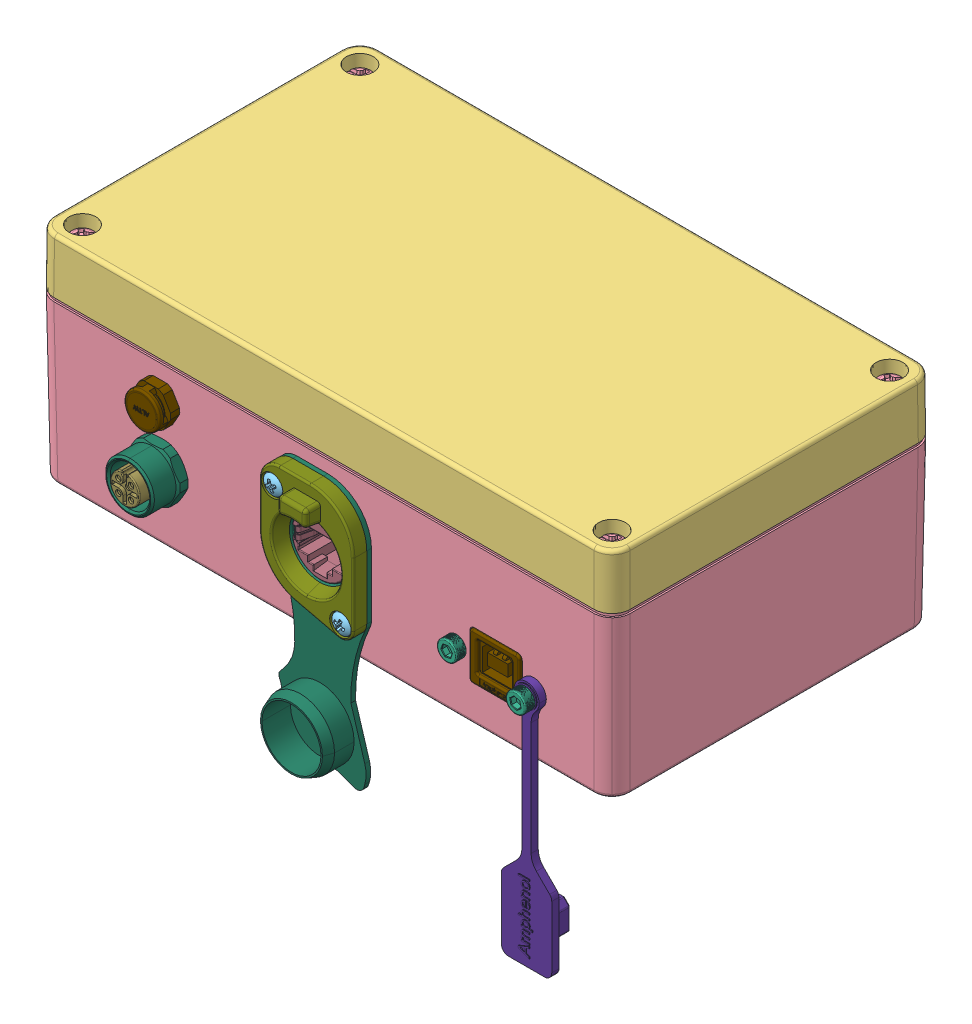
SolidWorks assembly Fleet-Monitor_V1.0, configuration Standard. Lengths in mm. (continued)
Components (placement in the parent): (continued)
- U2-1: U2 [Standard] x (1 0 0) z (0 1 0) size (12.85 11.2 5.9)
  - R1SX-1: R1SX [Standard] at (-21 29.5 0.35) x (-1 0 0) z (0 1 0) size (12.85 5.9 11.2)
- U5-1: U5 [Standard] x (1 0 0) z (0 1 0) size (9 9 1.6)
  - User Library-LQFP48_Grid_0_5-1: User Library-LQFP48_Grid_0_5 [Standard] at (-26.5351 -3.898 0) x (1 0 0) z (0 -1 0) size (9 1.6 9)
    - User Library-LQFP48_Grid_0.5_LQFP_PIN_2-1: User Library-LQFP48_Grid_0.5_LQFP_PIN_2 [Standard] at (4.5 0 0.25) x (0 0 -1) z (1 0 0) size (0.27 0.97 1.5)
    - User Library-LQFP48_Grid_0.5_LQFP_PIN_2-2: User Library-LQFP48_Grid_0.5_LQFP_PIN_2 [Standard] at (4.5 0 -1.25) x (0 0 -1) z (1 0 0) size (0.27 0.97 1.5)
    - User Library-LQFP48_Grid_0.5_LQFP_PIN_2-3: User Library-LQFP48_Grid_0.5_LQFP_PIN_2 [Standard] at (-4.5 0 2.75) x (0 0 1) z (-1 0 0) size (0.27 0.97 1.5)
    - User Library-LQFP48_Grid_0.5_LQFP_PIN_2-4: User Library-LQFP48_Grid_0.5_LQFP_PIN_2 [Standard] at (-4.5 0 1.75) x (0 0 1) z (-1 0 0) size (0.27 0.97 1.5)
    - User Library-LQFP48_Grid_0.5_LQFP_PIN_2-5: User Library-LQFP48_Grid_0.5_LQFP_PIN_2 [Standard] at (-0.75 0 4.5) size (0.27 0.97 1.5)
    - User Library-LQFP48_Grid_0.5_LQFP_PIN_2-6: User Library-LQFP48_Grid_0.5_LQFP_PIN_2 [Standard] at (4.5 0 2.25) x (0 0 -1) z (1 0 0) size (0.27 0.97 1.5)
    - User Library-LQFP48_Grid_0.5_LQFP_PIN_2-7: User Library-LQFP48_Grid_0.5_LQFP_PIN_2 [Standard] at (4.5 0 1.75) x (0 0 -1) z (1 0 0) size (0.27 0.97 1.5)
    - User Library-LQFP48_Grid_0.5_LQFP_PIN_2-8: User Library-LQFP48_Grid_0.5_LQFP_PIN_2 [Standard] at (2.75 0 -4.5) x (-1 0 0) z (0 0 -1) size (0.27 0.97 1.5)
    - User Library-LQFP48_Grid_0.5_LQFP_PIN_2-9: User Library-LQFP48_Grid_0.5_LQFP_PIN_2 [Standard] at (-4.5 0 -0.75) x (0 0 1) z (-1 0 0) size (0.27 0.97 1.5)
    - User Library-LQFP48_Grid_0.5_LQFP_PIN_2-10: User Library-LQFP48_Grid_0.5_LQFP_PIN_2 [Standard] at (4.5 0 0.75) x (0 0 -1) z (1 0 0) size (0.27 0.97 1.5)
    - User Library-LQFP48_Grid_0.5_LQFP_PIN_2-11: User Library-LQFP48_Grid_0.5_LQFP_PIN_2 [Standard] at (-1.75 0 -4.5) x (-1 0 0) z (0 0 -1) size (0.27 0.97 1.5)
    - User Library-LQFP48_Grid_0.5_LQFP_PIN_2-12: User Library-LQFP48_Grid_0.5_LQFP_PIN_2 [Standard] at (0.75 0 -4.5) x (-1 0 0) z (0 0 -1) size (0.27 0.97 1.5)
    - User Library-LQFP48_Grid_0.5_LQFP_PIN_2-13: User Library-LQFP48_Grid_0.5_LQFP_PIN_2 [Standard] at (-4.5 0 1.25) x (0 0 1) z (-1 0 0) size (0.27 0.97 1.5)
    - User Library-LQFP48_Grid_0.5_LQFP_PIN_2-14: User Library-LQFP48_Grid_0.5_LQFP_PIN_2 [Standard] at (4.5 0 -0.75) x (0 0 -1) z (1 0 0) size (0.27 0.97 1.5)
    - User Library-LQFP48_Grid_0.5_LQFP_PIN_2-15: User Library-LQFP48_Grid_0.5_LQFP_PIN_2 [Standard] at (-4.5 0 -1.25) x (0 0 1) z (-1 0 0) size (0.27 0.97 1.5)
    - User Library-LQFP48_Grid_0.5_LQFP_PIN_2-16: User Library-LQFP48_Grid_0.5_LQFP_PIN_2 [Standard] at (-0.25 0 4.5) size (0.27 0.97 1.5)
    - User Library-LQFP48_Grid_0.5_LQFP_PIN_2-17: User Library-LQFP48_Grid_0.5_LQFP_PIN_2 [Standard] at (-4.5 0 0.75) x (0 0 1) z (-1 0 0) size (0.27 0.97 1.5)
    - User Library-LQFP48_Grid_0.5_LQFP_PIN_2-18: User Library-LQFP48_Grid_0.5_LQFP_PIN_2 [Standard] at (-1.25 0 -4.5) x (-1 0 0) z (0 0 -1) size (0.27 0.97 1.5)
    - User Library-LQFP48_Grid_0.5_LQFP_PIN_2-19: User Library-LQFP48_Grid_0.5_LQFP_PIN_2 [Standard] at (-2.25 0 -4.5) x (-1 0 0) z (0 0 -1) size (0.27 0.97 1.5)
    - User Library-LQFP48_Grid_0.5_LQFP_PIN_2-20: User Library-LQFP48_Grid_0.5_LQFP_PIN_2 [Standard] at (-4.5 0 -1.75) x (0 0 1) z (-1 0 0) size (0.27 0.97 1.5)
    - User Library-LQFP48_Grid_0.5_LQFP_PIN_2-21: User Library-LQFP48_Grid_0.5_LQFP_PIN_2 [Standard] at (1.75 0 -4.5) x (-1 0 0) z (0 0 -1) size (0.27 0.97 1.5)
    - User Library-LQFP48_Grid_0.5_LQFP_PIN_2-22: User Library-LQFP48_Grid_0.5_LQFP_PIN_2 [Standard] at (0.25 0 -4.5) x (-1 0 0) z (0 0 -1) size (0.27 0.97 1.5)
    - User Library-LQFP48_Grid_0.5_LQFP_PIN_2-23: User Library-LQFP48_Grid_0.5_LQFP_PIN_2 [Standard] at (4.5 0 -2.25) x (0 0 -1) z (1 0 0) size (0.27 0.97 1.5)
    - User Library-LQFP48_Grid_0.5_LQFP_PIN_2-24: User Library-LQFP48_Grid_0.5_LQFP_PIN_2 [Standard] at (4.5 0 -2.75) x (0 0 -1) z (1 0 0) size (0.27 0.97 1.5)
    - User Library-LQFP48_Grid_0.5_LQFP_PIN_2-25: User Library-LQFP48_Grid_0.5_LQFP_PIN_2 [Standard] at (1.25 0 -4.5) x (-1 0 0) z (0 0 -1) size (0.27 0.97 1.5)
    - User Library-LQFP48_Grid_0.5_LQFP_PIN_2-26: User Library-LQFP48_Grid_0.5_LQFP_PIN_2 [Standard] at (1.25 0 4.5) size (0.27 0.97 1.5)
    - User Library-LQFP48_Grid_0.5_LQFP_PIN_2-27: User Library-LQFP48_Grid_0.5_LQFP_PIN_2 [Standard] at (-4.5 0 -2.25) x (0 0 1) z (-1 0 0) size (0.27 0.97 1.5)
    - User Library-LQFP48_Grid_0.5_LQFP_PIN_2-28: User Library-LQFP48_Grid_0.5_LQFP_PIN_2 [Standard] at (-1.25 0 4.5) size (0.27 0.97 1.5)
    - User Library-LQFP48_Grid_0.5_LQFP_PIN_2-29: User Library-LQFP48_Grid_0.5_LQFP_PIN_2 [Standard] at (-4.5 0 -0.25) x (0 0 1) z (-1 0 0) size (0.27 0.97 1.5)
    - User Library-LQFP48_Grid_0.5_LQFP_PIN_2-30: User Library-LQFP48_Grid_0.5_LQFP_PIN_2 [Standard] at (2.75 0 4.5) size (0.27 0.97 1.5)
    - User Library-LQFP48_Grid_0.5_LQFP_PIN_2-31: User Library-LQFP48_Grid_0.5_LQFP_PIN_2 [Standard] at (1.75 0 4.5) size (0.27 0.97 1.5)
    - User Library-LQFP48_Grid_0.5_LQFP_PIN_2-32: User Library-LQFP48_Grid_0.5_LQFP_PIN_2 [Standard] at (2.25 0 -4.5) x (-1 0 0) z (0 0 -1) size (0.27 0.97 1.5)
    - User Library-LQFP48_Grid_0.5_LQFP_PIN_2-33: User Library-LQFP48_Grid_0.5_LQFP_PIN_2 [Standard] at (4.5 0 2.75) x (0 0 -1) z (1 0 0) size (0.27 0.97 1.5)
    - User Library-LQFP48_Grid_0.5_LQFP_PIN_2-34: User Library-LQFP48_Grid_0.5_LQFP_PIN_2 [Standard] at (2.25 0 4.5) size (0.27 0.97 1.5)
    - User Library-LQFP48_Grid_0.5_LQFP_PIN_2-35: User Library-LQFP48_Grid_0.5_LQFP_PIN_2 [Standard] at (-2.25 0 4.5) size (0.27 0.97 1.5)
    - User Library-LQFP48_Grid_0.5_LQFP_PIN_2-36: User Library-LQFP48_Grid_0.5_LQFP_PIN_2 [Standard] at (-4.5 0 0.25) x (0 0 1) z (-1 0 0) size (0.27 0.97 1.5)
    - User Library-LQFP48_Grid_0.5_LQFP_PIN_2-37: User Library-LQFP48_Grid_0.5_LQFP_PIN_2 [Standard] at (-1.75 0 4.5) size (0.27 0.97 1.5)
    - User Library-LQFP48_Grid_0.5_LQFP_PIN_2-38: User Library-LQFP48_Grid_0.5_LQFP_PIN_2 [Standard] at (-4.5 0 -2.75) x (0 0 1) z (-1 0 0) size (0.27 0.97 1.5)
    - User Library-LQFP48_Grid_0.5_LQFP_PIN_2-39: User Library-LQFP48_Grid_0.5_LQFP_PIN_2 [Standard] at (-0.25 0 -4.5) x (-1 0 0) z (0 0 -1) size (0.27 0.97 1.5)
    - User Library-LQFP48_Grid_0.5_LQFP_PIN_2-40: User Library-LQFP48_Grid_0.5_LQFP_PIN_2 [Standard] at (4.5 0 1.25) x (0 0 -1) z (1 0 0) size (0.27 0.97 1.5)
    - User Library-LQFP48_Grid_0.5_LQFP_PIN_2-41: User Library-LQFP48_Grid_0.5_LQFP_PIN_2 [Standard] at (0.75 0 4.5) size (0.27 0.97 1.5)
    - User Library-LQFP48_Grid_0.5_LQFP_PIN_2-42: User Library-LQFP48_Grid_0.5_LQFP_PIN_2 [Standard] at (0.25 0 4.5) size (0.27 0.97 1.5)
    - User Library-LQFP48_Grid_0.5_LQFP_PIN_2-43: User Library-LQFP48_Grid_0.5_LQFP_PIN_2 [Standard] at (-0.75 0 -4.5) x (-1 0 0) z (0 0 -1) size (0.27 0.97 1.5)
    - User Library-LQFP48_Grid_0.5_LQFP_PIN_2-44: User Library-LQFP48_Grid_0.5_LQFP_PIN_2 [Standard] at (-4.5 0 2.25) x (0 0 1) z (-1 0 0) size (0.27 0.97 1.5)
    - User Library-LQFP48_Grid_0.5_LQFP_PIN_2-45: User Library-LQFP48_Grid_0.5_LQFP_PIN_2 [Standard] at (4.5 0 -0.25) x (0 0 -1) z (1 0 0) size (0.27 0.97 1.5)
    - User Library-LQFP48_Grid_0.5_LQFP_PIN_2-46: User Library-LQFP48_Grid_0.5_LQFP_PIN_2 [Standard] at (4.5 0 -1.75) x (0 0 -1) z (1 0 0) size (0.27 0.97 1.5)
    - User Library-LQFP48_Grid_0.5_LQFP_PIN_2-47: User Library-LQFP48_Grid_0.5_LQFP_PIN_2 [Standard] at (-2.75 0 -4.5) x (-1 0 0) z (0 0 -1) size (0.27 0.97 1.5)
    - User Library-LQFP48_Grid_0.5_LQFP_PIN_2-48: User Library-LQFP48_Grid_0.5_LQFP_PIN_2 [Standard] at (-2.75 0 4.5) size (0.27 0.97 1.5)
    - User Library-LQFP48_Grid_0.5_LQFP48_Koerper_2-1: User Library-LQFP48_Grid_0.5_LQFP48_Koerper_2 [Standard] at origin size (7 1.45 7)
- U7-1: U7 [Standard] x (1 0 0) z (0 1 0) size (2 2 0.95)
  - User Library-lga-2x2x0_9-1: User Library-lga-2x2x0_9 [Standard] at (27.75 0 0) size (2 2 0.95)
- C3-1: C3 [Standard] x (1 0 0) z (0 1 0) size (0.81 1.61 0.81)
  - C3-subassembly-1-1: C3-subassembly-1 [Standard] at (49.9999 -16.2499 0) x (0 1 0) z (0 0 1) size (1.61 0.81 0.81)
    - User Library-0603_Cap-1: User Library-0603_Cap [Standard] at origin size (0.41 0.81 0.81)
    - User Library-0603_Cap-1-1: User Library-0603_Cap-1 [Standard] at origin size (0.8 0.8 0.81)
    - User Library-0603_Cap-2-1: User Library-0603_Cap-2 [Standard] at origin size (0.41 0.81 0.81)
- C9-1: C9 [Standard] x (1 0 0) z (0 1 0) size (0.81 1.61 0.81)
  - C9-subassembly-1-1: C9-subassembly-1 [Standard] at (-28.4999 34.2499 0) x (0 -1 0) z (0 0 1) size (1.61 0.81 0.81)
    - User Library-0603_Cap-1: User Library-0603_Cap [Standard] at origin size (0.41 0.81 0.81)
    - User Library-0603_Cap-1-1: User Library-0603_Cap-1 [Standard] at origin size (0.8 0.8 0.81)
    - User Library-0603_Cap-2-1: User Library-0603_Cap-2 [Standard] at origin size (0.41 0.81 0.81)
- C17-1: C17 [Standard] x (1 0 0) z (0 1 0) size (1.61 0.81 0.81)
  - C17-subassembly-1-1: C17-subassembly-1 [Standard] at (-24.4999 -9.7499 0) x (1 0 0) z (0 0 1) size (1.61 0.81 0.81)
    - User Library-0603_Cap-1: User Library-0603_Cap [Standard] at origin size (0.41 0.81 0.81)
    - User Library-0603_Cap-1-1: User Library-0603_Cap-1 [Standard] at origin size (0.8 0.8 0.81)
    - User Library-0603_Cap-2-1: User Library-0603_Cap-2 [Standard] at origin size (0.41 0.81 0.81)
- C26-1: C26 [Standard] x (1 0 0) z (0 1 0) size (0.81 1.61 0.81)
  - C26-subassembly-1-1: C26-subassembly-1 [Standard] at (-2.5001 -18.9999 0) x (0 1 0) z (0 0 1) size (1.61 0.81 0.81)
    - User Library-0603_Cap-1: User Library-0603_Cap [Standard] at origin size (0.41 0.81 0.81)
    - User Library-0603_Cap-1-1: User Library-0603_Cap-1 [Standard] at origin size (0.8 0.8 0.81)
    - User Library-0603_Cap-2-1: User Library-0603_Cap-2 [Standard] at origin size (0.41 0.81 0.81)
- L3-1: L3 [Standard] x (1 0 0) z (0 1 0) size (2 1.2 0.95)
  - User Library-ind_0805-1: User Library-ind_0805 [Standard] at (-26.7501 21.7499 0) x (-1 0 0) z (0 0 1) size (2 1.2 0.95)
- R15-1: R15 [Standard] x (1 0 0) z (0 1 0) size (1.6 0.82 0.45)
  - User Library-Panasonic0603-1: User Library-Panasonic0603 [Standard] at (3.0001 -21.7499 0) x (-1 0 0) z (0 0 1) size (1.6 0.82 0.45)
- R16-1: R16 [Standard] x (1 0 0) z (0 1 0) size (1.6 0.82 0.45)
  - User Library-Panasonic0603-1: User Library-Panasonic0603 [Standard] at (0.2501 -20.9999 0) x (-1 0 0) z (0 0 1) size (1.6 0.82 0.45)
- R17-1: R17 [Standard] x (1 0 0) z (0 1 0) size (1.6 0.82 0.45)
  - User Library-Panasonic0603-1: User Library-Panasonic0603 [Standard] at (3.0001 -20.2499 0) x (-1 0 0) z (0 0 1) size (1.6 0.82 0.45)
- R22-1: R22 [Standard] x (1 0 0) z (0 1 0) size (1.6 0.82 0.45)
  - User Library-Panasonic0603-1: User Library-Panasonic0603 [Standard] at (0.2501 -15.7499 0) x (-1 0 0) z (0 0 1) size (1.6 0.82 0.45)
- R23-1: R23 [Standard] x (1 0 0) z (0 1 0) size (1.6 0.82 0.45)
  - User Library-Panasonic0603-1: User Library-Panasonic0603 [Standard] at (3.0001 -16.4999 0) x (-1 0 0) z (0 0 1) size (1.6 0.82 0.45)
- R25-1: R25 [Standard] x (1 0 0) z (0 1 0) size (0.82 1.6 0.45)
  - User Library-Panasonic0603-1: User Library-Panasonic0603 [Standard] at (-4.9999 -19.0001 0) x (0 1 0) z (0 0 1) size (1.6 0.82 0.45)
- R26-1: R26 [Standard] x (1 0 0) z (0 1 0) size (0.82 1.6 0.45)
  - User Library-Panasonic0603-1: User Library-Panasonic0603 [Standard] at (-3.7499 -19.0001 0) x (0 1 0) z (0 0 1) size (1.6 0.82 0.45)
- S2-1: S2 [Standard] x (1 0 0) z (0 1 0) size (6.4 5.1 1.5)
  - S2-subassembly-1-1: S2-subassembly-1 [Standard] at (14.2499 27.2499 0) x (-1 0 0) z (0 1 0) size (6.4 1.5 5.1)
    - User Library-LP16-1: User Library-LP16 [Standard] at origin size (4.8 0.65 4.8)
    - User Library-LP16-1-1: User Library-LP16-1 [Standard] at origin size (1.45 0.35 0.5)
    - User Library-LP16-2-1: User Library-LP16-2 [Standard] at origin size (2 0.7 2)
    - User Library-LP16-3-1: User Library-LP16-3 [Standard] at origin size (1.45 0.35 0.5)
    - User Library-LP16-4-1: User Library-LP16-4 [Standard] at origin size (5.1 1.16 5.1)
    - User Library-LP16-5-1: User Library-LP16-5 [Standard] at origin size (1.45 0.35 0.5)
    - User Library-LP16-6-1: User Library-LP16-6 [Standard] at origin size (1.45 0.35 0.5)
- X5-1: X5 [Standard] x (1 0 0) z (0 1 0) size (12.7 6.1 5.46)
  - SHF_105_01_L_D_SM-1: SHF_105_01_L_D_SM [Standard] at (60.9601 -16.3999 0.12) x (1 0 0) z (0 -1 0) size (12.7 5.46 6.1)
    - _T_1S71_02_05_D_SM_6-1: _T_1S71_02_05_D_SM_6 [Standard] at origin size (5.49 4.83 6.1)
    - _SHF_First_Position_Indicator_4-1: _SHF_First_Position_Indicator_4 [Standard] at (-2.54 5.334 2.54) size (1.02 1.27 0.25)
    - _SHF_105_01_D_header_2-1: _SHF_105_01_D_header_2 [Standard] at origin size (12.7 5.33 5.59)
- X4-1: X4 [Standard] x (1 0 0) z (0 1 0) size (26 40.83 70.74)
  - NE8FDH-C5E-TOP-1: NE8FDH-C5E-TOP [Standard] at (-0.0001 -46.0551 12.5) x (1 0 0) z (0 -1 0) size (26 33.72 34.8)
    - NE8FDH-C5E-TOP-subassembly-1-1: NE8FDH-C5E-TOP-subassembly-1 [Standard] at origin size (26 33.72 26.34)
      - ne8fdh body-1: ne8fdh body [Standard] at origin size (2.2 8.85 2.47)
      - ne8fdh body-1-1: ne8fdh body-1 [Standard] at origin size (26 31 26.34)
    - NE8FDH-C5E-TOP-subassembly-2-1: NE8FDH-C5E-TOP-subassembly-2 [Standard] at origin size (25.5 29.75 12.56)
      - pcb-1-1: pcb-1 [Standard] at origin size (0.64 0.64 0.8)
      - pcb-2-1: pcb-2 [Standard] at origin size (0.64 0.63 0.8)
      - pcb-3-1: pcb-3 [Standard] at origin size (0.64 0.63 0.8)
      - pcb-4-1: pcb-4 [Standard] at origin size (0.64 0.64 0.8)
      - pcb-5-1: pcb-5 [Standard] at origin size (0.64 0.64 0.8)
      - pcb-6-1: pcb-6 [Standard] at origin size (0.63 0.63 0.8)
      - pcb-7-1: pcb-7 [Standard] at origin size (0.63 0.63 0.8)
      - pcb-8-1: pcb-8 [Standard] at origin size (0.63 0.63 0.8)
      - pcb-9-1: pcb-9 [Standard] at origin size (0.64 0.63 1.6)
      - pcb-10-1: pcb-10 [Standard] at origin size (0.64 0.63 1.6)
      - pcb-11-1: pcb-11 [Standard] at origin size (0.64 0.64 1.6)
      - pcb-12-1: pcb-12 [Standard] at origin size (0.64 0.64 1.6)
      - pcb-13-1: pcb-13 [Standard] at origin size (0.63 0.63 1.6)
      - pcb-14-1: pcb-14 [Standard] at origin size (0.63 0.63 1.6)
      - pcb-15-1: pcb-15 [Standard] at origin size (0.63 0.63 1.6)
      - pcb-16-1: pcb-16 [Standard] at origin size (0.64 0.64 1.6)
      - pcb-17-1: pcb-17 [Standard] at origin size (25.5 26.35 1.6)
      - pcb-18-1: pcb-18 [Standard] at origin size (2.84 21.54 10.16)
      - pcb-19-1: pcb-19 [Standard] at origin size (2.84 21.54 10.17)
  - rubber seal-1: rubber seal [Standard] at (0 -44.8001 12.5) x (1 0 0) z (0 -1 0) size (26 70.74 10.4)
  - NE8FDH-C5E-TOP_Flange-1: NE8FDH-C5E-TOP_Flange [Standard] at (0 -44.8001 12.5) x (1 0 0) z (0 -1 0) size (26 33.1 8.03)
- X3-1: X3 [Standard] x (1 0 0) z (0 1 0) size (32 20.25 74.01)
  - M-MUSB-D111-31-REVT1_Rubber-1: M-MUSB-D111-31-REVT1_Rubber [Standard] at (58.4999 -47.25 -48.5) x (1 0 0) z (0 -1 0) size (14 68.5 8.25)
  - M-MUSB-D111-31-REVT1_Body-1: M-MUSB-D111-31-REVT1_Body [Standard] at (22.5 -41.7501 5.5) x (1 0 0) z (0 -1 0) size (28 18 18)
- X2-1: X2 [Standard] x (1 0 0) z (0 1 0) size (5.61 12.65 13.08)
  - X2-subassembly-1-1: X2-subassembly-1 [Standard] at (-51.5 31.7501 5) x (0 1 0) z (0 0 1) size (12.65 5.61 13.08)
    - 436500315-1: 436500315 [Standard] at origin size (2.6 1.2 2.45)
    - 436500315-1-1: 436500315-1 [Standard] at origin size (12.65 4.4 13.08)
- J1-1: J1 [Standard] x (1 0 0) z (0 1 0) size (5.08 2.54 11.78)
  - J1-subassembly-1-1: J1-subassembly-1 [Standard] at (-44.25 36.5001 0) x (-1 0 0) z (0 0 1) size (5.08 2.54 11.78)
    - Jumper Closed-1: Jumper Closed [Standard] at origin size (5.08 2.54 11.39)
    - Jumper Closed-1-1: Jumper Closed-1 [Standard] at origin size (4.99 2.45 5.98)
- P3-1: P3 [Standard] x (1 0 0) z (0 1 0) size (0.73 1.65 0.68)
  - P3-subassembly-1-1: P3-subassembly-1 [Standard] at (-24.4001 -32.4249 0) x (-1 0 0) z (0 0 1) size (0.72 1.65 0.68)
    - User Library-LED SMD0603-1: User Library-LED SMD0603 [Standard] at origin size (0.65 0.28 0.35)
    - User Library-LED SMD0603-1-1: User Library-LED SMD0603-1 [Standard] at origin size (0.65 0.28 0.35)
    - User Library-LED SMD0603-2-1: User Library-LED SMD0603-2 [Standard] at origin size (0.15 0.16 0.07)
    - User Library-LED SMD0603-3-1: User Library-LED SMD0603-3 [Standard] at origin size (0.72 1 0.35)
    - User Library-LED SMD0603-4-1: User Library-LED SMD0603-4 [Standard] at origin size (0.72 1.6 0.3)
- P4-1: P4 [Standard] x (1 0 0) z (0 1 0) size (0.73 1.65 0.68)
  - P4-subassembly-1-1: P4-subassembly-1 [Standard] at (-29.4001 -32.4249 0) x (-1 0 0) z (0 0 1) size (0.72 1.65 0.68)
    - User Library-LED SMD0603-1: User Library-LED SMD0603 [Standard] at origin size (0.65 0.28 0.35)
    - User Library-LED SMD0603-1-1: User Library-LED SMD0603-1 [Standard] at origin size (0.65 0.28 0.35)
    - User Library-LED SMD0603-2-1: User Library-LED SMD0603-2 [Standard] at origin size (0.15 0.16 0.07)
    - User Library-LED SMD0603-3-1: User Library-LED SMD0603-3 [Standard] at origin size (0.72 1 0.35)
    - User Library-LED SMD0603-4-1: User Library-LED SMD0603-4 [Standard] at origin size (0.72 1.6 0.3)
- R27-1: R27 [Standard] x (1 0 0) z (0 1 0) size (3.2 1.6 0.52)
  - User Library-R-0603-Array-4-1-1: User Library-R-0603-Array-4-1 [Standard] at (47.2501 -16.2502 0) x (1 0 0) z (0 0 1) size (3.2 1.6 0.52)
- R28-1: R28 [Standard] x (1 0 0) z (0 1 0) size (1.6 3.2 0.52)
  - User Library-R-0603-Array-4-1-1: User Library-R-0603-Array-4-1 [Standard] at (35.2498 -0.7501 0) x (0 -1 0) z (0 0 1) size (3.2 1.6 0.52)
- X1-1: X1 [Standard] x (1 0 0) z (0 1 0) size (19.5 26 19.6)
  - T4145015021-001 Plastic-1: T4145015021-001 Plastic [Standard] at (-45.0001 -55.3001 8.5) x (1 0 0) z (0 -1 0) size (19.5 19.1 26)
    - T4145015021-001 Plastic-subassembly-1-1: T4145015021-001 Plastic-subassembly-1 [Standard] at (0 0 -16) x (0 0 1) z (0 1 0) size (16 15.2 13.25)
      - Front Plastic-1: Front Plastic [Standard] at origin size (2 5.1 3)
      - Front Plastic-1-1: Front Plastic-1 [Standard] at origin size (2 5.1 3)
      - Front Plastic-2-1: Front Plastic-2 [Standard] at origin size (16 9.5 9.5)
    - Back Plastic-1: Back Plastic [Standard] at origin size (19.5 19.1 10)
  - Inside Nut-1: Inside Nut [Standard] at (-45.0001 -2.98 8.5) x (0 -1 0) z (0 0 1) size (7.8 17.27 15)
  - Outside Nut-1: Outside Nut [Standard] at (-45.0001 -12.7999 8.5) x (0 -1 0) z (0 0 1) size (9.54 15 14.06)
- U3-1: U3 [Standard] x (1 0 0) z (0 1 0) size (5 6.24 1.75)
  - User Library-SO-8-1-1: User Library-SO-8-1 [Standard] at (-34.2673 18.7499 0) x (-1 0 0) z (0 0 1) size (5 6.24 1.75)
- U4-1: U4 [Standard] x (1 0 0) z (0 1 0) size (6.24 5 1.75)
  - User Library-SO-8-1-1: User Library-SO-8-1 [Standard] at (-33.2501 31.5173 0) x (0 1 0) z (0 0 1) size (5 6.24 1.75)
- Board-1: Board [Standard] x (1 0 0) z (0 1 0) size (140.5 79.5 1.6)
  - Board-Part-1-1: Board-Part-1 [Standard] at (0 0 -1.5986) size (140.5 79.5 1.6)
- VENT-PS2XXX-XXXXX-1: VENT-PS2XXX-XXXXX [Standard] at (-52.4385 27.8739 38.1824) x (0 -0.01309 0.999914) z (-0.43221 0.901696 0.011804) size (12.37 10.27 10.75)
- nut_gb_t_808_m6x0_75-1: nut_gb_t_808_m6x0_75 [Default] at (-45.0001 25.0207 41.8763) x (0 0.01309 -0.999914) z (0 0.999914 0.01309) size (2.4 11.55 10)
- U6-subassembly-11-1: U6-subassembly-11 [Standard] at (-6.1951 1.05 -6.345) x (0 0 1) z (0 1 0) size (12.69 12.39 3.97)
- Case Lid-1: Case Lid [Standard] at (-67.276 34 -32.873) x (1 0 0) z (0 0 1) size (160 15.53 90)
- Case Screw-1: Case Screw [Standard] at (-126.9366 34 -9.222) x (0.598788 0 -0.800908) z (0.800908 0 0.598788) size (6.8 22.2 6.8)
- Case Screw-2: Case Screw [Standard] at (-67.276 34 -109.873) x (1 0 0) z (0 0 1) size (6.8 22.2 6.8)
- Case Screw-3: Case Screw [Standard] at (79.724 34 -32.873) x (1 0 0) z (0 0 1) size (6.8 22.2 6.8)
- Case Screw-4: Case Screw [Standard] at (15.2047 34 -80.1476) x (0.508431 0 -0.861103) z (0.861103 0 0.508431) size (6.8 22.2 6.8)
- SCREW-1: SCREW [Default] at (-9.5 24.5 40.5626) x (0.927966 0.372665 0) z (0 0 1) size (5.56 5.56 9.97)
- SCREW-2: SCREW [Default] at (9.5 0.5 40.5626) x (0.951461 -0.307769 0) z (0 0 1) size (5.56 5.56 9.97)
- M3x10.step-1: M3x10.step [Standard] at (36.4999 6.4409 44.633) x (0.981312 0.192405 0.002519) z (0 -0.01309 0.999914) size (5.5 5.5 12.8)
- M3x10.step-2: M3x10.step [Standard] at (58.4999 6.4029 47.5328) x (0.750234 0.661115 0.008655) z (0 -0.01309 0.999914) size (5.5 5.5 12.8)
- 436450300-1: 436450300 [Standard] at (-51.525 13.95 -31.7051) x (0 0 1) z (-1 0 0) size (9.85 14 7.21)
- Wire_1-1: Wire_1 [Standard] at (-57.0709 17.1292 -4.0542) x (0.922073 -0.005043 0.386984) z (-0.380187 0.175209 0.908163) size (40.42 17.32 36.45)
- Wire_2-1: Wire_2 [Standard] at (-58.0329 10.2224 -2.8387) x (0.918571 0.262436 0.295558) z (-0.387637 0.744253 0.543898) size (40.15 37.67 22.03)
- Wire_3-1: Wire_3 [Standard] at (-56.9966 11.4516 4.055) x (0.925543 -0.270145 0.265314) z (-0.371225 -0.509395 0.776343) size (35.85 19.35 45.51)
- c-929967-1-a2-3d.stp-1: c-929967-1-a2-3d.stp [Standard] at (-95.6676 16.624 -4.0542) x (0.000171 -0.013088 0.999914) z (-0.999914 -0.01309 0) size (7.17 5.38 34.12)
- c-929967-1-a2-3d.stp-2: c-929967-1-a2-3d.stp [Standard] at (-95.6835 17.8394 2.8394) x (0.000171 -0.013088 0.999914) z (-0.999914 -0.01309 0) size (7.17 5.38 34.12)
- c-929967-1-a2-3d.stp-3: c-929967-1-a2-3d.stp [Standard] at (-95.5774 9.7309 -2.8387) x (0.000171 -0.013088 0.999914) z (-0.999914 -0.01309 0) size (7.17 5.38 34.12)
- c-929967-1-a2-3d.stp-4: c-929967-1-a2-3d.stp [Standard] at (-95.5933 10.9463 4.055) x (0.000171 -0.013088 0.999914) z (-0.999914 -0.01309 0) size (7.17 5.38 34.12)
- c-0965687-01-b-3d_Ring.step-1: c-0965687-01-b-3d_Ring.step [Standard] at (-79.7316 13.9933 0.0004) x (0.000171 -0.013088 -0.999914) z (0.999914 0.01309 0) size (33.6 33.72 9.01)
Mates (geometry in assembly coordinates):
- Abstand1: distance = 0.5 mm anti-aligned: plane of VENT-PS2XXX-XXXXX-1 through (-45.0001 24.9749 45.3757) normal (0 0.01309 -0.999914); plane of Free-Models-1/1554J-Body-1/1554J.stp-1/1554J Box.stp-1 through (-80 34.5 45.0004) normal (0 -0.01309 0.999914)
- Konzentrisch1: concentric aligned: cylinder of Free-Models-1/1554J-Body-1/1554J.stp-1/1554J Box.stp-1 through (-45.0001 25.1124 34.8766) axis (0 -0.01309 0.999914) radius 2.6; cylinder of VENT-PS2XXX-XXXXX-1 through (-45.0001 24.9422 47.8755) axis (0 -0.01309 0.999914) radius 4.9
- Parallel3: parallel aligned: line of Free-Models-1/1554J-Body-1/1554J.stp-1/1554J Box.stp-1 through (-74.4243 -10.5 43.4243) axis (1 0 0); line of VENT-PS2XXX-XXXXX-1 through (-46.9726 19.9426 47.81) axis (1 0 0)
- Konzentrisch2: concentric anti-aligned: circle of Free-Models-1/1554J-Body-1/1554J.stp-1/1554J Box.stp-1; circle of nut_gb_t_808_m6x0_75-1
- Deckungsgleich4: coincident anti-aligned: plane of Free-Models-1/1554J-Body-1/1554J.stp-1/1554J Box.stp-1 through (-64.5 34.5 42.0004) normal (0 0.01309 -0.999914); plane of nut_gb_t_808_m6x0_75-1 through (-48.0073 25.0207 41.8763) normal (0 -0.01309 0.999914)
- Parallel4: parallel aligned: line of Free-Models-1/1554J-Body-1/1554J.stp-1/1554J Box.stp-1 through (64.5 34.5 42.0004) axis (-1 0 0); line of nut_gb_t_808_m6x0_75-1 through (-42.1133 30.0203 41.9417) axis (-1 0 0)
- Deckungsgleich5: coincident: plane of U6-1/U6-subassembly-1-1/RPMB-3.0-35-1 through (-6.1951 -6.345 1.015) normal (-1 0 0); plane of U6-subassembly-11-1 through (-6.1951 1.015 6.345) normal (-1 0 0)
- Deckungsgleich6: coincident: plane of U6-1/U6-subassembly-1-1/RPMB-3.0-1 through (5.0499 -5.85 1.05) normal (0 -1 0); plane of U6-subassembly-11-1 through (5.0499 1.05 5.85) normal (0 0 1)
- Deckungsgleich7: coincident aligned: plane of U6-1/U6-subassembly-1-1/RPMB-3.0-35-1 through (-6.1951 6.345 1.015) normal (0 0 1); plane of U6-subassembly-11-1 through (-6.1951 1.015 -6.345) normal (0 1 0)
- Konzentrisch3: concentric anti-aligned: cylinder of Free-Models-1/1554J-Body-1/1554J.stp-1/IN-M4 (insert M4-0.7X5.75mm SS).stp-3 through (73.5 23.5015 38.5004) axis (0 1 0) radius 1.6256; cone of Case Lid-1 through (73.5 49.5 38.5004) axis (0 -1 0)
- Konzentrisch4: concentric anti-aligned: cylinder of Free-Models-1/1554J-Body-1/1554J.stp-1/IN-M4 (insert M4-0.7X5.75mm SS).stp-1 through (-73.5 23.5015 -38.4996) axis (0 1 0) radius 1.6256; cone of Case Lid-1 through (-73.5 49.5 -38.4996) axis (0 -1 0)
- Tangential3: tangent: plane of Free-Models-1/1554J-Body-1/1554J.stp-1/1554J Box.stp-1 through (0 34.5 0.0004) normal (0 1 0); curve of Case Lid-1
- Konzentrisch5: concentric aligned: cone of Case Lid-1 through (-73.5 49.5 -38.4996) axis (0 -1 0); cylinder of Case Screw-2 through (-73.5 34.7 -38.4996) axis (0 -1 0) radius 1.94
- Konzentrisch6: concentric aligned: cone of Case Lid-1 through (73.5 49.5 38.5004) axis (0 -1 0); cylinder of Case Screw-3 through (73.5 34.7 38.5004) axis (0 -1 0) radius 1.94
- Deckungsgleich13: coincident anti-aligned: plane of Case Lid-1 through (-73.5 44.5 -38.4996) normal (0 1 0); plane of Case Screw-2 through (-73.5 44.5 -40.4396) normal (0 -1 0)
- Deckungsgleich14: coincident anti-aligned: plane of Case Lid-1 through (73.5 44.5 38.5004) normal (0 1 0); plane of Case Screw-3 through (73.5 44.5 36.5604) normal (0 -1 0)
- Konzentrisch7: concentric aligned: cone of Case Lid-1 through (-73.5 49.5 38.5004) axis (0 -1 0); cylinder of Case Screw-1 through (-73.5 34.7 38.5004) axis (0 -1 0) radius 1.94
- Deckungsgleich15: coincident anti-aligned: plane of Case Lid-1 through (-73.5 44.5 38.5004) normal (0 1 0); plane of Case Screw-1 through (-75.0538 44.5 37.3387) normal (0 -1 0)
- Konzentrisch9: concentric aligned: cone of Case Lid-1 through (73.5 49.5 -38.4996) axis (0 -1 0); cylinder of Case Screw-4 through (73.5 34.7 -38.4996) axis (0 -1 0) radius 1.94
- Deckungsgleich16: coincident anti-aligned: plane of Case Lid-1 through (73.5 44.5 -38.4996) normal (0 1 0); circle of Case Screw-4
- Konzentrisch10: concentric anti-aligned: cylinder of X4-1/NE8FDH-C5E-TOP_Flange-1 through (-9.5 24.5 49.9001) axis (0 0 1) radius 3; cylinder of SCREW-1 through (-9.5 24.5 49.3415) axis (0 0 -1) radius 2.7813
- Konzentrisch12: concentric anti-aligned: cylinder of X4-1/NE8FDH-C5E-TOP_Flange-1 through (9.5 0.5 49.9001) axis (0 0 1) radius 3; cylinder of SCREW-2 through (9.5 0.5 49.3414) axis (0 0 -1) radius 2.7813
- Deckungsgleich17: coincident anti-aligned: circle of X4-1/NE8FDH-C5E-TOP_Flange-1; plane of SCREW-1 through (-6.3206 23.1425 48.5001) normal (0 0 -1)
- Deckungsgleich18: coincident: point of X4-1/NE8FDH-C5E-TOP_Flange-1; plane of SCREW-2 through (11.0735 -2.5782 48.5001) normal (0 0 -1)
- Konzentrisch13: concentric anti-aligned: cylinder of Free-Models-1/1554J-Body-1/1554J.stp-1/1554J Box.stp-1 through (36.4999 6.5718 34.6339) axis (0 -0.01309 0.999914) radius 1.6; circle of M3x10.step-1
- Deckungsgleich19: coincident anti-aligned: plane of Free-Models-1/1554J-Body-1/1554J.stp-1/1554J Box.stp-1 through (-80 34.5 45.0004) normal (0 -0.01309 0.999914); plane of M3x10.step-1 through (36.4999 6.4409 44.633) normal (0 0.01309 -0.999914)
- Konzentrisch14: concentric aligned: cylinder of Free-Models-1/1554J-Body-1/1554J.stp-1/1554J Box.stp-1 through (58.4999 6.5718 34.6339) axis (0 -0.01309 0.999914) radius 1.6; circle of M3x10.step-2
- Abstand2: distance = 2.9 mm anti-aligned: plane of M3x10.step-2 through (58.4999 6.4029 47.5328) normal (0 0.01309 -0.999914); plane of Free-Models-1/1554J-Body-1/1554J.stp-1/1554J Box.stp-1 through (-80 34.5 45.0004) normal (0 -0.01309 0.999914)
- Parallel7: parallel aligned: plane of X2-1/X2-subassembly-1-1/436500315-1-1 through (-53.43 0.05 -25.4251) normal (-1 0 0); plane of 436450300-1 through (-53.475 17.6 -36.6251) normal (-1 0 0)
- Deckungsgleich24: coincident anti-aligned: plane of X2-1/X2-subassembly-1-1/436500315-1-1 through (-52.77 9.95 -27.4801) normal (1 0 0); plane of 436450300-1 through (-52.77 9.95 -29.9301) normal (-1 0 0)
- Deckungsgleich25: coincident anti-aligned: plane of X2-1/X2-subassembly-1-1/436500315-1-1 through (-53.43 9.95 -25.4251) normal (0 1 0); plane of 436450300-1 through (-53.475 9.95 -36.6251) normal (0 -1 0)
- Deckungsgleich27: coincident anti-aligned: plane of X2-1/X2-subassembly-1-1/436500315-1-1 through (-50.93 9.95 -27.4801) normal (0 0 -1); plane of 436450300-1 through (-52.77 9.95 -27.4801) normal (0 0 1)
- Konzentrisch15: concentric anti-aligned: circle of Free-Models-1/c-1-967402-1-d2-3d_Receptacle-1; circle of Wire_1-1
- Deckungsgleich28: coincident anti-aligned: plane of Free-Models-1/c-1-967402-1-d2-3d_Receptacle-1 through (-57.0709 17.1292 -4.0542) normal (0.999914 0.01309 0); plane of Wire_1-1 through (-57.0709 17.1292 -4.0542) normal (-0.999914 -0.01309 0)
- Konzentrisch16: concentric anti-aligned: circle of Free-Models-1/c-1-967402-1-d2-3d_Receptacle-1; circle of Wire_2-1
- Deckungsgleich29: coincident anti-aligned: plane of Free-Models-1/c-1-967402-1-d2-3d_Receptacle-1 through (-56.9807 10.2361 -2.8387) normal (0.999914 0.01309 0); plane of Wire_2-1 through (-56.9807 10.2361 -2.8387) normal (-0.999914 -0.01309 0)
- Konzentrisch17: concentric anti-aligned: circle of Free-Models-1/c-1-967402-1-d2-3d_Receptacle-1; circle of Wire_3-1
- Deckungsgleich30: coincident anti-aligned: plane of Wire_3-1 through (-56.9966 11.4516 4.055) normal (-0.999914 -0.01309 0); plane of Free-Models-1/c-1-967402-1-d2-3d_Receptacle-1 through (-56.9966 11.4516 4.055) normal (0.999914 0.01309 0)
- Konzentrisch18: concentric anti-aligned: cylinder of Free-Models-1/c-1-967402-1-d2-3d_Receptacle-1 through (-88.0933 16.7231 -4.0542) axis (0.999914 0.01309 0) radius 2.25; cylinder of c-929967-1-a2-3d.stp-1 through (-64.3803 17.0335 -4.0542) axis (-0.999914 -0.01309 0) radius 1.245
- Deckungsgleich31: coincident aligned: plane of Free-Models-1/c-1-967402-1-d2-3d_Receptacle-1 through (-85.5685 16.7562 -4.0542) normal (-0.999914 -0.01309 0); plane of c-929967-1-a2-3d.stp-1 through (-85.5685 16.7562 -4.0542) normal (-0.999914 -0.01309 0)
- Konzentrisch19: concentric anti-aligned: cylinder of Free-Models-1/c-1-967402-1-d2-3d_Receptacle-1 through (-88.1092 17.9385 2.8394) axis (0.999914 0.01309 0) radius 2.25; cylinder of c-929967-1-a2-3d.stp-2 through (-64.3962 18.249 2.8394) axis (-0.999914 -0.01309 0) radius 1.245
- Konzentrisch20: concentric anti-aligned: cylinder of Free-Models-1/c-1-967402-1-d2-3d_Receptacle-1 through (-88.003 9.83 -2.8387) axis (0.999914 0.01309 0) radius 2.25; cylinder of c-929967-1-a2-3d.stp-3 through (-64.2901 10.1405 -2.8387) axis (-0.999914 -0.01309 0) radius 1.245
- Konzentrisch21: concentric anti-aligned: cylinder of Free-Models-1/c-1-967402-1-d2-3d_Receptacle-1 through (-88.019 11.0455 4.055) axis (0.999914 0.01309 0) radius 2.25; cylinder of c-929967-1-a2-3d.stp-4 through (-64.306 11.3559 4.055) axis (-0.999914 -0.01309 0) radius 1.245
- Deckungsgleich32: coincident aligned: plane of Free-Models-1/c-1-967402-1-d2-3d_Receptacle-1 through (-85.5844 17.9716 2.8394) normal (-0.999914 -0.01309 0); plane of c-929967-1-a2-3d.stp-2 through (-85.5844 17.9716 2.8394) normal (-0.999914 -0.01309 0)
- Deckungsgleich33: coincident aligned: plane of Free-Models-1/c-1-967402-1-d2-3d_Receptacle-1 through (-85.4942 11.0785 4.055) normal (-0.999914 -0.01309 0); plane of c-929967-1-a2-3d.stp-4 through (-85.4942 11.0785 4.055) normal (-0.999914 -0.01309 0)
- Deckungsgleich34: coincident aligned: plane of Free-Models-1/c-1-967402-1-d2-3d_Receptacle-1 through (-85.4783 9.8631 -2.8387) normal (-0.999914 -0.01309 0); plane of c-929967-1-a2-3d.stp-3 through (-85.4783 9.8631 -2.8387) normal (-0.999914 -0.01309 0)
- Konzentrisch22: concentric anti-aligned: cylinder of Free-Models-1/c-1-967402-1-d2-3d_Receptacle-1 through (-102.2299 13.6987 0.0004) axis (0.999914 0.01309 0) radius 13.3; cylinder of c-0965687-01-b-3d_Ring.step-1 through (-79.2816 13.9992 0.0004) axis (-0.999914 -0.01309 0) radius 13.4
- Deckungsgleich35: coincident anti-aligned: plane of Free-Models-1/1554J-Body-1/1554J.stp-1/1554J Box.stp-1 through (-80 34.5 -44.9996) normal (-0.999914 -0.01309 0); plane of c-0965687-01-b-3d_Ring.step-1 through (-79.7316 13.9933 0.0004) normal (0.999914 0.01309 0)
